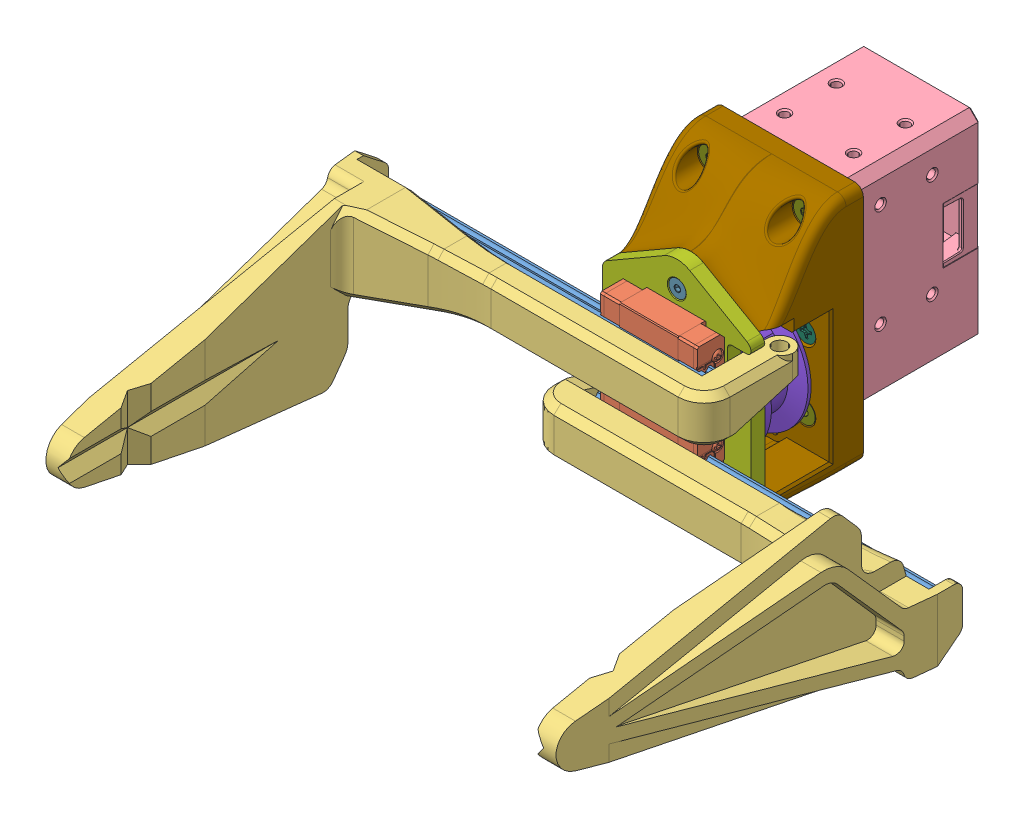
SolidWorks assembly Gripper_Assy, configuration Default. Lengths in mm.
Overall size (135.15 64.73 143.19).
29 component instances, 17 part files, 61 mates.
Components (placement in the parent):
- Gripper_Geo-1: Gripper_Geo [Default] at origin size (140.5 320.38 611.55) (hidden)
- MGN7_Rail-1: MGN7_Rail [80mm] at (24.4268 9 485.409) x (0 1 0) z (-1 0 0) size (7 4.8 80)
- MGN7_Rail-2: MGN7_Rail [80mm] at (75.5732 -9 485.409) x (0 1 0) z (-1 0 0) size (7 4.8 80)
- MGN7C_Carriage-1: MGN7C_Carriage [Default] at (0 9 482.959) x (0 -1 0) z (1 0 0) size (17 6.5 23.48)
- MGN7C_Carriage-2: MGN7C_Carriage [Default] at (0 -9 482.959) x (0 -1 0) z (1 0 0) size (17 6.5 23.48)
- Gripper_Jaw-1: Gripper_Jaw [Default] at (2.6768 0 0.1) size (88 34.92 96.64)
- Gripper_Jaw-2: Gripper_Jaw [Default] at (-2.6768 0 0.1) x (-1 0 0) z (0 0 1) size (88 34.92 96.64)
- XM430-1: XM430 [Default] at (0 0 440.709) x (-1 0 0) z (0 0 1) size (28.5 46.5 34)
- XC430_Horn-1: XC430_Horn [Default] at (0 0 442.209) x (-0.461728 0.887021 0) z (0 0 1) size (20.5 20.5 5.4)
- 9293K111_Constant-Force Spring-1: 9293K111_Constant-Force Spring [9293K111] at (0 20.4659 473.1591) x (0 0 1) z (0 -1 0) size (4.75 11.59 8.52)
- Gripper_Carriage_Mount-1: Gripper_Carriage_Mount [Default] at origin size (34.5 52.93 3.17)
- Gripper_Drive_Pulley-1: Gripper_Drive_Pulley [Default] at (0 0 1.5) x (0.999857 -0.016895 0) z (0 0 1) size (29.31 29.31 13.21)
- Gripper_Structure-1: Gripper_Structure [Default] at origin size (34.93 64.73 22.83)
- CF_Spring_Idler-1: CF_Spring_Idler [Default] at (11.3305 3.4226 0) x (0.832765 0.553627 0) z (0 0 1) size (8.62 8.62 6.75)
- CF_Spring_Idler-2: CF_Spring_Idler [Default] at (13.8894 -35.4971 0) x (0.734452 0.678661 0) z (0 0 1) size (8.62 8.62 6.75)
- 91292A831_18-8 Stainless Steel Socket Head Screw-1: 91292A831_18-8 Stainless Steel Socket Head Screw [91292A831] at (55.5732 -9 491.309) x (-0.599094 -0.800678 0) z (0 0 1) size (3.8 3.8 8.1)
- 91292A835_18-8 Stainless Steel Socket Head Screw-1: 91292A835_18-8 Stainless Steel Socket Head Screw [91292A835] at (0.1352 7.9989 458.4182) x (-0.923728 -0.383049 0) z (0 0 -1) size (3.8 3.8 16.14)
- 92125A051_18-8 Stainless Steel Hex Drive Flat Head Screw-1: 92125A051_18-8 Stainless Steel Hex Drive Flat Head Screw [92125A051] at (-4 15 479.174) x (-1 0 0) z (0 0 -1) size (4 4 5.21)
- 92125A059_18-8 Stainless Steel Hex Drive Flat Head Screw-1: 92125A059_18-8 Stainless Steel Hex Drive Flat Head Screw [92125A059] at (0 20.4659 471.569) size (4 4 16.28)
- 92010A775_Passivated 18-8 Stainless Steel Phillips Flat Head Screw-1: 92010A775_Passivated 18-8 Stainless Steel Phillips Flat Head Screw [92010A775] at (-11 8 459.309) size (4.7 4.7 6.14)
- 92125A085_18-8 Stainless Steel Hex Drive Flat Head Screw-1: 92125A085_18-8 Stainless Steel Hex Drive Flat Head Screw [92125A085] at (-11 32 461.139) size (5 5 16.3)
- 92125A085_18-8 Stainless Steel Hex Drive Flat Head Screw-2: 92125A085_18-8 Stainless Steel Hex Drive Flat Head Screw [92125A085] at (11 32 461.139) x (0.987351 0.158553 0) z (0 0 1) size (5 5 16.3)
- 92125A085_18-8 Stainless Steel Hex Drive Flat Head Screw-4: 92125A085_18-8 Stainless Steel Hex Drive Flat Head Screw [92125A085] at (11 -8 461.139) x (0.959125 0.282984 0) z (0 0 1) size (5 5 16.3)
- 92125A085_18-8 Stainless Steel Hex Drive Flat Head Screw-6: 92125A085_18-8 Stainless Steel Hex Drive Flat Head Screw [92125A085] at (-11 -8 461.139) x (0.928571 0.371154 0) z (0 0 1) size (5 5 16.3)
- 92010A775_Passivated 18-8 Stainless Steel Phillips Flat Head Screw-2: 92010A775_Passivated 18-8 Stainless Steel Phillips Flat Head Screw [92010A775] at (11 8 459.309) x (0.987351 0.158553 0) z (0 0 1) size (4.7 4.7 6.14)
- 92125A059_18-8 Stainless Steel Hex Drive Flat Head Screw-2: 92125A059_18-8 Stainless Steel Hex Drive Flat Head Screw [92125A059] at (0 -20.4659 471.569) x (0.987351 0.158553 0) z (0 0 1) size (4 4 16.28)
- 91292A835_18-8 Stainless Steel Socket Head Screw-2: 91292A835_18-8 Stainless Steel Socket Head Screw [91292A835] at (7.9989 -0.1352 458.4182) x (-0.85131 -0.524663 0) z (0 0 -1) size (3.8 3.8 16.14)
- 91292A835_18-8 Stainless Steel Socket Head Screw-3: 91292A835_18-8 Stainless Steel Socket Head Screw [91292A835] at (-0.1352 -7.9989 458.4182) x (-0.777574 -0.628792 0) z (0 0 -1) size (3.8 3.8 16.14)
- 91292A835_18-8 Stainless Steel Socket Head Screw-4: 91292A835_18-8 Stainless Steel Socket Head Screw [91292A835] at (-7.9989 0.1352 458.4182) x (-0.715577 -0.698533 0) z (0 0 -1) size (3.8 3.8 16.14)
Mates (geometry in assembly coordinates):
- Width1: width anti-aligned: plane of MGN7C_Carriage-1 through (6.75 12.5 482.959) normal (0 -1 0); plane of MGN7_Rail-1 through (6.75 5.5 482.959) normal (0 1 0); plane of MGN7C_Carriage-1 through (-75.5732 12.5 483.7152) normal (0 1 0); plane of MGN7_Rail-1 through (-75.5732 5.5 483.7152) normal (0 -1 0)
- Coincident7: coincident anti-aligned: plane of MGN7_Rail-1 through (-75.5732 5.7 483.009) normal (0 0 -1); plane of MGN7C_Carriage-1 through (6.75 9 483.009) normal (0 0 1)
- Coincident8: coincident: line of Gripper_Geo-1 through (-11.25 17.5 479.709) axis (0 -1 0); plane of MGN7C_Carriage-1 through (-11.25 9 482.959) normal (-1 0 0)
- Coincident9: coincident anti-aligned: plane of Gripper_Geo-1 through (0 0 479.709) normal (0 0 1); plane of MGN7C_Carriage-1 through (6.75 9 479.709) normal (0 0 -1)
- Coincident11: coincident: line of Gripper_Geo-1 through (11.25 17.5 479.709) axis (-1 0 0); plane of MGN7C_Carriage-1 through (6.75 17.5 482.959) normal (0 1 0)
- Coincident12: coincident: line of Gripper_Geo-1 through (-11.25 -17.5 479.709) axis (1 0 0); plane of MGN7C_Carriage-2 through (6.75 -17.5 482.959) normal (0 -1 0)
- Coincident13: coincident: line of Gripper_Geo-1 through (11.25 -0.5 479.709) axis (0 -1 0); plane of MGN7C_Carriage-2 through (11.25 -9 482.959) normal (1 0 0)
- Coincident14: coincident anti-aligned: plane of Gripper_Geo-1 through (0 0 479.709) normal (0 0 1); plane of MGN7C_Carriage-2 through (6.75 -9 479.709) normal (0 0 -1)
- Coincident15: coincident anti-aligned: plane of MGN7_Rail-2 through (-24.4268 -12.3 483.009) normal (0 0 -1); plane of MGN7C_Carriage-2 through (6.75 -9 483.009) normal (0 0 1)
- Width2: width anti-aligned: plane of MGN7_Rail-2 through (-24.4268 -12.5 483.7152) normal (0 -1 0); plane of MGN7C_Carriage-2 through (-24.4268 -5.5 483.7152) normal (0 1 0); plane of MGN7_Rail-2 through (6.75 -12.5 482.959) normal (0 1 0); plane of MGN7C_Carriage-2 through (6.75 -5.5 482.959) normal (0 -1 0)
- Coincident16: coincident: line of Gripper_Geo-1 through (-11.75 -5.5 457.709) axis (0 -1 0); plane of MGN7_Rail-2 through (-11.75 -12.5 465.809) normal (-1 0 0)
- Coincident17: coincident: line of Gripper_Geo-1 through (11.75 12.5 457.709) axis (0 -1 0); plane of MGN7_Rail-1 through (11.75 5.5 465.809) normal (1 0 0)
- Linear/Linear Coupler1: linear coupler = 0.001 : 0.001 mm: plane of MGN7_Rail-1 through (-65.5732 5.5 487.809) normal (-1 0 0); plane of MGN7_Rail-2 through (65.5732 -12.5 487.809) normal (1 0 0)
- Coincident18: coincident anti-aligned: plane of Gripper_Geo-1 through (0 0 479.709) normal (0 0 1); plane of MGN7C_Carriage-3 through (0 6.425 479.709) normal (0 0 -1)
- Coincident20: coincident: line of Gripper_Geo-1 through (11.25 3.175 479.709) axis (-1 0 0); plane of MGN7C_Carriage-3 through (-6.75 3.175 479.709) normal (0 -1 0)
- Coincident21: coincident: line of Gripper_Geo-1 through (11.25 9.675 479.709) axis (0 -1 0); plane of MGN7C_Carriage-3 through (11.25 6.425 479.709) normal (1 0 0)
- Coincident35: coincident anti-aligned: plane of MGN7_Rail-1 through (-65.5732 5.5 487.809) normal (-1 0 0); plane of Gripper_Jaw-1 through (-65.5732 0 0.1) normal (1 0 0)
- Coincident36: coincident anti-aligned: plane of MGN7_Rail-1 through (-75.5732 5.7 487.809) normal (0 0 1); plane of Gripper_Jaw-1 through (-60.3232 0 487.809) normal (0 0 -1)
- Coincident37: coincident anti-aligned: plane of MGN7_Rail-2 through (65.5732 -12.5 487.809) normal (1 0 0); plane of Gripper_Jaw-2 through (65.5732 0 0.1) normal (-1 0 0)
- Coincident38: coincident anti-aligned: plane of MGN7_Rail-2 through (-24.4268 -12.3 487.809) normal (0 0 1); plane of Gripper_Jaw-2 through (60.3232 0 487.809) normal (0 0 -1)
- Concentric3: concentric aligned: line of XM430-1 through (0 0 422.0076) axis (0 0 1); cylinder of XC430_Horn-1 through (0 0 457.709) axis (0 0 1) radius 10.25
- Coincident39: coincident anti-aligned: plane of XM430-1 through (-12.0843 -10.85 457.709) normal (0 0 1); plane of XC430_Horn-1 through (0 0 457.709) normal (0 0 -1)
- Coincident40: coincident aligned: line of Gripper_Geo-1 through (0 0 353.5534) axis (0 0 1); line of XM430-1 through (0 0 422.0076) axis (0 0 1)
- Concentric4: concentric aligned: cylinder of Gripper_Geo-1 through (0 20.4659 476.534) axis (0 0 1) radius 2.1365; circle of 9293K111_Constant-Force Spring-1
- Parallel1: parallel: plane of Gripper_Geo-1 through (4.81 18.2321 469.7842) normal (0 -1 0); line of 9293K111_Constant-Force Spring-1 through (0 16.6559 473.1591) axis (1 0 0)
- Width5: width aligned: plane of 9293K111_Constant-Force Spring-1 through (-1.3031 16.8857 475.534) normal (0 0 1); plane of Gripper_Geo-1 through (-1.3031 16.8857 470.7842) normal (0 0 -1); plane of 9293K111_Constant-Force Spring-1 through (0 22.1159 476.034) normal (0 0 1); plane of Gripper_Geo-1 through (0 24.7759 470.2842) normal (0 0 -1)
- Coincident41: coincident anti-aligned: plane of Gripper_Geo-1 through (0 0 457.709) normal (0 0 -1); plane of XM430-1 through (-12.0843 -10.85 457.709) normal (0 0 1)
- Concentric5: concentric aligned: cylinder of Gripper_Geo-1 through (-11 -8 461.209) axis (0 0 1) radius 1.35; cylinder of XM430-1 through (-11 -8 457.709) axis (0 0 1) radius 2.4
- LimitDistance1: limit distance = 50.1386 mm: plane of MGN7C_Carriage-1 through (11.25 9 482.959) normal (1 0 0); plane of MGN7_Rail-1 through (14.4268 5.5 487.809) normal (1 0 0)
- Concentric7: concentric aligned: cylinder of MGN7_Rail-1 through (-55.5732 9 487.81) axis (0 0 -1) radius 1.2; cylinder of Gripper_Jaw-1 through (-55.5732 9 498.4759) axis (0 0 -1) radius 1.65
- Coincident42: coincident anti-aligned: plane of MGN7C_Carriage-1 through (6.75 9 479.709) normal (0 0 -1); plane of Gripper_Carriage_Mount-1 through (0 -20.4659 479.709) normal (0 0 1)
- Concentric8: concentric aligned: cylinder of MGN7C_Carriage-1 through (4 15 479.709) axis (0 0 -1) radius 0.8; cylinder of Gripper_Carriage_Mount-1 through (4 15 476.534) axis (0 0 -1) radius 1.1
- Concentric9: concentric aligned: cylinder of MGN7C_Carriage-1 through (-4 15 479.709) axis (0 0 -1) radius 0.8; cylinder of Gripper_Carriage_Mount-1 through (-4 15 476.534) axis (0 0 -1) radius 1.1
- Coincident44: coincident anti-aligned: plane of Gripper_Carriage_Mount-1 through (0 -20.4659 476.534) normal (0 0 -1); plane of Gripper_Structure-1 through (0 20.4659 476.534) normal (0 0 1)
- Concentric11: concentric aligned: cylinder of Gripper_Carriage_Mount-1 through (0 20.4659 479.709) axis (0 0 1) radius 1.1; cylinder of Gripper_Structure-1 through (0 20.4659 462.7842) axis (0 0 1) radius 1.65
- Concentric12: concentric aligned: cylinder of Gripper_Carriage_Mount-1 through (0 -20.4659 479.709) axis (0 0 1) radius 1.1; cylinder of Gripper_Structure-1 through (0 -20.4659 462.7842) axis (0 0 1) radius 1.65
- Concentric13: concentric aligned: cylinder of Gripper_Carriage_Mount-1 through (0 20.4659 479.709) axis (0 0 1) radius 1.1; cylinder of CF_Spring_Idler-1 through (0 20.4659 476.534) axis (0 0 1) radius 2.1365
- Width6: width anti-aligned: plane of CF_Spring_Idler-1 through (-0.6367 21.4236 476.534) normal (0 0 1); plane of Gripper_Carriage_Mount-1 through (-0.9135 21.84 469.7842) normal (0 0 -1); plane of CF_Spring_Idler-1 through (0 -20.4659 476.534) normal (0 0 -1); plane of Gripper_Structure-1 through (0 20.4659 469.7842) normal (0 0 1)
- Concentric14: concentric aligned: cylinder of Gripper_Carriage_Mount-1 through (0 -20.4659 479.709) axis (0 0 1) radius 1.1; cylinder of CF_Spring_Idler-2 through (0 -20.4659 476.534) axis (0 0 1) radius 2.1365
- Width7: width anti-aligned: plane of CF_Spring_Idler-2 through (-0.7805 -19.6213 476.534) normal (0 0 1); plane of Gripper_Structure-1 through (-1.1198 -19.2541 469.7842) normal (0 0 -1); plane of CF_Spring_Idler-2 through (0 -20.4659 469.7842) normal (0 0 1); plane of Gripper_Carriage_Mount-1 through (0 -20.4659 476.534) normal (0 0 -1)
- Concentric15: concentric aligned: cylinder of MGN7_Rail-2 through (55.5732 -9 487.81) axis (0 0 -1) radius 1.2; cylinder of Gripper_Jaw-2 through (55.5732 -9 498.4759) axis (0 0 -1) radius 1.65
- LimitDistance2: limit distance = 54.3232 mm aligned: plane of MGN7_Rail-2 through (65.5732 -12.5 487.809) normal (1 0 0); plane of MGN7C_Carriage-2 through (11.25 -9 482.959) normal (1 0 0)
- Coincident47: coincident aligned: cone of Gripper_Structure-1 through (-11 8 461.209) axis (0 0 -1); cone of 92010A775_Passivated 18-8 Stainless Steel Phillips Flat Head Screw-1 through (-11 8 459.759) axis (0 0 -1)
- Coincident48: coincident aligned: cone of Gripper_Carriage_Mount-1 through (-4 15 476.534) axis (0 0 1); cone of 92125A051_18-8 Stainless Steel Hex Drive Flat Head Screw-1 through (-4 15 476.734) axis (0 0 1)
- Concentric17: concentric aligned: circle of MGN7_Rail-2; circle of 91292A831_18-8 Stainless Steel Socket Head Screw-1
- Coincident49: coincident anti-aligned: plane of MGN7_Rail-2 through (55.5732 -9 485.309) normal (0 0 -1); plane of 91292A831_18-8 Stainless Steel Socket Head Screw-1 through (55.5732 -9 485.309) normal (0 0 1)
- Coincident50: coincident aligned: cone of Gripper_Carriage_Mount-1 through (0 20.4659 479.709) axis (0 0 -1); cone of 92125A059_18-8 Stainless Steel Hex Drive Flat Head Screw-1 through (0 20.4659 479.509) axis (0 0 -1)
- Coincident51: coincident aligned: cone of Gripper_Structure-1 through (-11 32 461.209) axis (0 0 -1); cone of 92125A085_18-8 Stainless Steel Hex Drive Flat Head Screw-1 through (-11 32 459.709) axis (0 0 -1)
- Coincident52: coincident aligned: cone of Gripper_Structure-1 through (11 32 461.209) axis (0 0 -1); cone of 92125A085_18-8 Stainless Steel Hex Drive Flat Head Screw-2 through (11 32 459.709) axis (0 0 -1)
- Coincident53: coincident aligned: cone of Gripper_Structure-1 through (11 -8 461.209) axis (0 0 -1); cone of 92125A085_18-8 Stainless Steel Hex Drive Flat Head Screw-4 through (11 -8 459.709) axis (0 0 -1)
- Coincident54: coincident aligned: cone of Gripper_Structure-1 through (-11 -8 461.209) axis (0 0 -1); cone of 92125A085_18-8 Stainless Steel Hex Drive Flat Head Screw-6 through (-11 -8 459.709) axis (0 0 -1)
- Coincident55: coincident aligned: cone of Gripper_Structure-1 through (11 8 461.209) axis (0 0 -1); cone of 92010A775_Passivated 18-8 Stainless Steel Phillips Flat Head Screw-2 through (11 8 459.759) axis (0 0 -1)
- Coincident56: coincident aligned: cone of Gripper_Carriage_Mount-1 through (0 -20.4659 479.709) axis (0 0 -1); cone of 92125A059_18-8 Stainless Steel Hex Drive Flat Head Screw-2 through (0 -20.4659 479.509) axis (0 0 -1)
- Coincident57: coincident anti-aligned: plane of Gripper_Drive_Pulley-1 through (1.235 7.9803 472.4182) normal (0 0 1); plane of 91292A835_18-8 Stainless Steel Socket Head Screw-1 through (0.1352 7.9989 472.4182) normal (0 0 -1)
- Concentric18: concentric anti-aligned: cylinder of Gripper_Drive_Pulley-1 through (0.1352 7.9989 474.4182) axis (0 0 1) radius 2.2; cylinder of 91292A835_18-8 Stainless Steel Socket Head Screw-1 through (0.1352 7.9989 474.4182) axis (0 0 -1) radius 1.9
- Coincident58: coincident anti-aligned: plane of Gripper_Drive_Pulley-1 through (1.235 7.9803 472.4182) normal (0 0 1); plane of 91292A835_18-8 Stainless Steel Socket Head Screw-2 through (7.9989 -0.1352 472.4182) normal (0 0 -1)
- Concentric19: concentric anti-aligned: cylinder of Gripper_Drive_Pulley-1 through (7.9989 -0.1352 474.4182) axis (0 0 1) radius 2.2; cylinder of 91292A835_18-8 Stainless Steel Socket Head Screw-2 through (7.9989 -0.1352 474.4182) axis (0 0 -1) radius 1.9
- Coincident59: coincident anti-aligned: plane of Gripper_Drive_Pulley-1 through (1.235 7.9803 472.4182) normal (0 0 1); plane of 91292A835_18-8 Stainless Steel Socket Head Screw-3 through (-0.1352 -7.9989 472.4182) normal (0 0 -1)
- Concentric20: concentric anti-aligned: cylinder of Gripper_Drive_Pulley-1 through (-0.1352 -7.9989 474.4182) axis (0 0 1) radius 2.2; cylinder of 91292A835_18-8 Stainless Steel Socket Head Screw-3 through (-0.1352 -7.9989 474.4182) axis (0 0 -1) radius 1.9
- Coincident60: coincident anti-aligned: plane of Gripper_Drive_Pulley-1 through (1.235 7.9803 472.4182) normal (0 0 1); plane of 91292A835_18-8 Stainless Steel Socket Head Screw-4 through (-7.9989 0.1352 472.4182) normal (0 0 -1)
- Concentric21: concentric anti-aligned: cylinder of Gripper_Drive_Pulley-1 through (-7.9989 0.1352 474.4182) axis (0 0 1) radius 2.2; cylinder of 91292A835_18-8 Stainless Steel Socket Head Screw-4 through (-7.9989 0.1352 474.4182) axis (0 0 -1) radius 1.9
